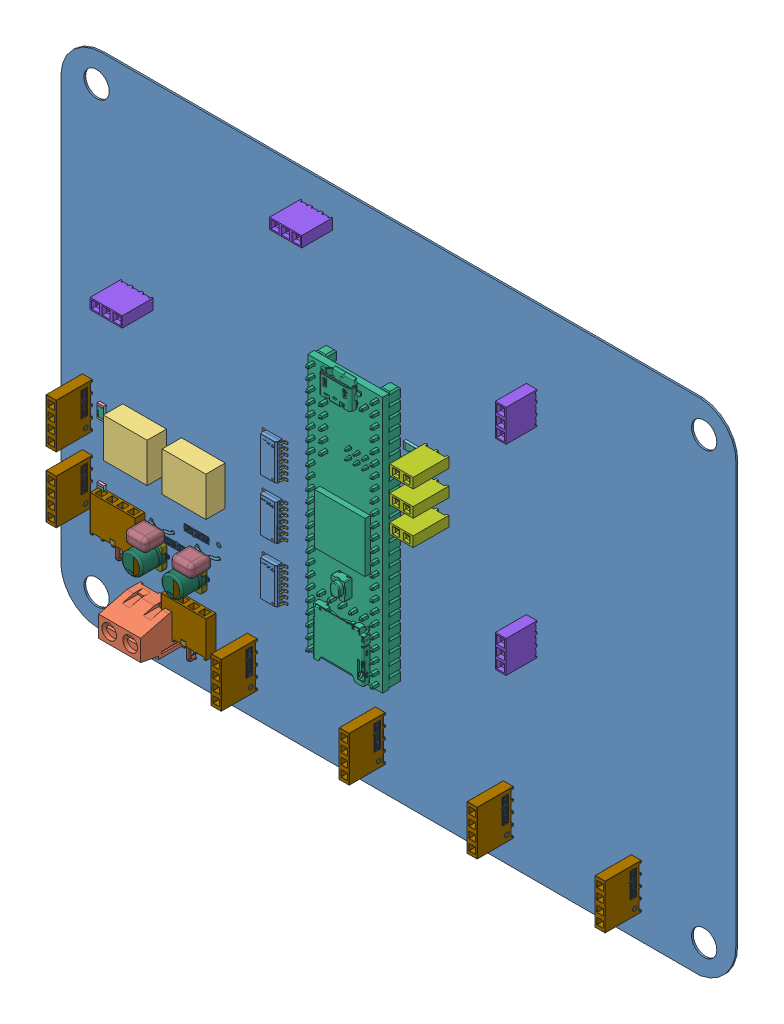
SolidWorks assembly MotherBoardPCB, configuration Default. Lengths in mm.
Overall size (160.64 119 16.7).
180 component instances, 26 part files, 0 mates.
Components (placement in the parent):
- MotherBoardPCB.step-1: MotherBoardPCB.step [Default] at origin size (160.64 119 16.7)
  - Board.step-1: Board.step [Default] at origin size (160.64 119 0.41)
    - Open CASCADE STEP translator 6.8 1.1.1.step-1: Open CASCADE STEP translator 6.8 1.1.1.step [Default] at (0 0 -0.4115) size (160.64 119 0.41)
  - J14.step-1: J14.step [Default] at origin size (10.6 8.2 13.5)
    - c-282836-2-h-3d.step-1: c-282836-2-h-3d.step [Default] at (49.784 31.8411 5) x (1 0 0) z (0 -1 0) size (10.6 13.5 8.2)
  - U6.step-1: U6.step [Default] at origin size (10.4 9.35 4.6)
    - 6221563216.step-1: 6221563216.step [Default] at (45.72 69.847 0) size (10.4 9.35 4.6)
      - Extruded.step-1: Extruded.step [Default] at origin size (10.4 9.35 4.6)
  - R5.step-1: R5.step [Default] at origin size (1.6 3.2 0.65)
    - Res_Samsung_RC3216F111CS_eec.step-1: Res_Samsung_RC3216F111CS_eec.step [Default] at (35.814 70.739 0) x (-1 0 0) z (0 0 1) size (1.6 3.2 0.65)
      - Sides.step-1: Sides.step [Default] at origin size (1.6 3.2 0.65)
      - Core.step-1: Core.step [Default] at origin size (1.6 3.14 0.59)
      - Top.step-1: Top.step [Default] at origin size (1.6 2.3 0.03)
      - Text_Logo.step-1: Text_Logo.step [Default] at (0.8 -1.12 0.65) size (0.2 1.32 0)
  - R4.step-1: R4.step [Default] at origin size (1.6 3.2 0.65)
    - Res_Samsung_RC3216F111CS_eec.step-1: Res_Samsung_RC3216F111CS_eec.step [Default] at (35.814 54.3773 0) x (-1 0 0) z (0 0 1) size (1.6 3.2 0.65)
      - Sides.step-1: Sides.step [Default] at origin size (1.6 3.2 0.65)
      - Core.step-1: Core.step [Default] at origin size (1.6 3.14 0.59)
      - Top.step-1: Top.step [Default] at origin size (1.6 2.3 0.03)
      - Text_Logo.step-1: Text_Logo.step [Default] at (0.8 -1.12 0.65) size (0.2 1.32 0)
  - J13.step-1: J13.step [Default] at origin size (2.41 10.67 11.41)
    - Conn_Samtec_SSW-104-01-G-S-003_eec.step-1: Conn_Samtec_SSW-104-01-G-S-003_eec.step [Default] at (32.131 70.612 0) x (0 1 0) z (0 0 1) size (10.67 2.41 11.41)
      - pins.step-1: pins.step [Default] at origin size (8.41 0.41 5.77)
      - body.step-1: body.step [Default] at origin size (10.67 2.41 8.64)
      - logo.step-1: logo.step [Default] at (-1.27 -1.205 4.32) x (1 0 0) z (0 -1 0) size (8.76 1.82 0)
  - J12.step-1: J12.step [Default] at origin size (2.41 10.67 11.41)
    - Conn_Samtec_SSW-104-01-G-S-003_eec.step-1: Conn_Samtec_SSW-104-01-G-S-003_eec.step [Default] at (32.131 54.991 0) x (0 1 0) z (0 0 1) size (10.67 2.41 11.41)
      - pins.step-1: pins.step [Default] at origin size (8.41 0.41 5.77)
      - body.step-1: body.step [Default] at origin size (10.67 2.41 8.64)
      - logo.step-1: logo.step [Default] at (-1.27 -1.205 4.32) x (1 0 0) z (0 -1 0) size (8.76 1.82 0)
  - D2.step-1: D2.step [Default] at origin size (10.67 12.15 6.58)
    - Diode_Vishay_UF4007-E3-54_eec.step-1: Diode_Vishay_UF4007-E3-54_eec.step [Default] at (40.64 48.641 0) x (1 0 0) z (0 0 1) size (10.67 12.15 6.58)
      - Lead.step-1: Lead.step [Default] at (0 5.438 -3.65) size (0.79 11.66 5.39)
      - body.step-1: body.step [Default] at (0 -2.325 1.35) x (1 0 0) z (0 1 0) size (10.67 2.41 8.64)
      - ring.step-1: ring.step [Default] at (0 -1.7813 1.35) x (0.981351 0 0.192225) z (0 1 0) size (2.7 2.7 1)
  - C4.step-1: C4.step [Default] at origin size (8.76 4.81 10.6)
    - Cap_Kemet_C322C104K5R5TA_eec.step-1: Cap_Kemet_C322C104K5R5TA_eec.step [Default] at (49.911 53.975 0) x (1 0 0) z (0 0 1) size (8.76 4.81 10.6)
      - Package.step-1: Package.step [Default] at origin size (5.09 3.19 4.82)
      - Leads.step-1: Leads.step [Default] at origin size (5.62 0.52 5.79)
      - logo.step-1: logo.step [Default] at origin size (8.76 1.82 0)
  - C3.step-1: C3.step [Default] at origin size (6 5.3 6.1)
    - Cap_Panasonic_Electronic_Components_EEE-FK1H100UR_eec.step-1: Cap_Panasonic_Electronic_Components_EEE-FK1H100UR_eec.step [Default] at (48.641 48.514 0) x (-1 0 0) z (0 0 1) size (6 5.3 6.1)
      - 5_SIZE_CODE_C.step-1: 5_SIZE_CODE_C.step [Default] x (1 0 0) z (0 -1 0) size (6 6.1 5.3)
        - __X2__2022__X0__W__X2__FFFD20AC__X0__SIZE_CODE_C-001.step-1: __X2__2022__X0__W__X2__FFFD20AC__X0__SIZE_CODE_C-001.step [Default] at (0 0.5 0) size (5 5.6 5)
        - __X2__2022__X0__W__X2__FFFD20AC__X0__SIZE_CODE_C-002.step-1: __X2__2022__X0__W__X2__FFFD20AC__X0__SIZE_CODE_C-002.step [Default] at origin size (5.3 1.15 5.3)
        - __X2__2022__X0__W__X2__FFFD20AC__X0__SIZE_CODE_C-003.step-1: __X2__2022__X0__W__X2__FFFD20AC__X0__SIZE_CODE_C-003.step [Default] at (-0.75 0.3 0) size (2.58 1 0.65)
        - __X2__2022__X0__W__X2__FFFD20AC__X0__SIZE_CODE_C-003.step-2: __X2__2022__X0__W__X2__FFFD20AC__X0__SIZE_CODE_C-003.step [Default] at (0.75 0.3 0) x (-1 0 0) z (0 0 -1) size (2.58 1 0.65)
        - 1.step-1: 1.step [Default] at (0 0.499 0) size (3.23 0.2 3.86)
  - U5.step-1: U5.step [Default] at origin size (6 8.65 1.76)
    - IC_Texas_Instruments_OPA4191IDR_eec.step-1: IC_Texas_Instruments_OPA4191IDR_eec.step [Default] at (76.868 56.769 0) x (-1 0 0) z (0 0 1) size (6 8.65 1.76)
      - IC_BODY.step-1: IC_BODY.step [Default] at (0 0 0.25) x (0 -1 0) z (0 0 1) size (8.65 3.9 1.5)
      - circle.step-1: circle.step [Default] at (-1.0199 3.7488 1.751) x (1 0 0) z (0 0 -1) size (0.4 0.4 0)
      - IC_LEG.step-1: IC_LEG.step [Default] at (-3 4.0195 0) x (1 0 0) z (0 -1 0) size (1.15 1.11 0.42)
      - IC_LEG.step-2: IC_LEG.step [Default] at (-3 2.7495 0) x (1 0 0) z (0 -1 0) size (1.15 1.11 0.42)
      - IC_LEG.step-3: IC_LEG.step [Default] at (-3 1.4795 0) x (1 0 0) z (0 -1 0) size (1.15 1.11 0.42)
      - IC_LEG.step-4: IC_LEG.step [Default] at (-3 0.2095 0) x (1 0 0) z (0 -1 0) size (1.15 1.11 0.42)
      - IC_LEG.step-5: IC_LEG.step [Default] at (-3 -1.0605 0) x (1 0 0) z (0 -1 0) size (1.15 1.11 0.42)
      - IC_LEG.step-6: IC_LEG.step [Default] at (-3 -2.3305 0) x (1 0 0) z (0 -1 0) size (1.15 1.11 0.42)
      - IC_LEG.step-7: IC_LEG.step [Default] at (-3 -3.6005 0) x (1 0 0) z (0 -1 0) size (1.15 1.11 0.42)
      - IC_LEG_MIR8.step-1: IC_LEG_MIR8.step [Default] at (3 4.0195 0) x (-1 0 0) z (0 1 0) size (1.15 1.11 0.42)
      - IC_LEG_MIR8.step-2: IC_LEG_MIR8.step [Default] at (3 2.7495 0) x (-1 0 0) z (0 1 0) size (1.15 1.11 0.42)
      - IC_LEG_MIR8.step-3: IC_LEG_MIR8.step [Default] at (3 1.4795 0) x (-1 0 0) z (0 1 0) size (1.15 1.11 0.42)
      - IC_LEG_MIR8.step-4: IC_LEG_MIR8.step [Default] at (3 0.2095 0) x (-1 0 0) z (0 1 0) size (1.15 1.11 0.42)
      - IC_LEG_MIR8.step-5: IC_LEG_MIR8.step [Default] at (3 -1.0605 0) x (-1 0 0) z (0 1 0) size (1.15 1.11 0.42)
      - IC_LEG_MIR8.step-6: IC_LEG_MIR8.step [Default] at (3 -2.3305 0) x (-1 0 0) z (0 1 0) size (1.15 1.11 0.42)
      - IC_LEG_MIR8.step-7: IC_LEG_MIR8.step [Default] at (3 -3.6005 0) x (-1 0 0) z (0 1 0) size (1.15 1.11 0.42)
      - Texas_Instruments.step-1: Texas_Instruments.step [Default] at (-0.0141 -3.2232 1.75) size (3.04 0.71 0.02)
  - U4.step-1: U4.step [Default] at origin size (6 8.65 1.76)
    - IC_Texas_Instruments_OPA4191IDR_eec.step-1: IC_Texas_Instruments_OPA4191IDR_eec.step [Default] at (76.835 69.85 0) x (-1 0 0) z (0 0 1) size (6 8.65 1.76)
      - IC_BODY.step-1: IC_BODY.step [Default] at (0 0 0.25) x (0 -1 0) z (0 0 1) size (8.65 3.9 1.5)
      - circle.step-1: circle.step [Default] at (-1.0199 3.7488 1.751) x (1 0 0) z (0 0 -1) size (0.4 0.4 0)
      - IC_LEG.step-1: IC_LEG.step [Default] at (-3 4.0195 0) x (1 0 0) z (0 -1 0) size (1.15 1.11 0.42)
      - IC_LEG.step-2: IC_LEG.step [Default] at (-3 2.7495 0) x (1 0 0) z (0 -1 0) size (1.15 1.11 0.42)
      - IC_LEG.step-3: IC_LEG.step [Default] at (-3 1.4795 0) x (1 0 0) z (0 -1 0) size (1.15 1.11 0.42)
      - IC_LEG.step-4: IC_LEG.step [Default] at (-3 0.2095 0) x (1 0 0) z (0 -1 0) size (1.15 1.11 0.42)
      - IC_LEG.step-5: IC_LEG.step [Default] at (-3 -1.0605 0) x (1 0 0) z (0 -1 0) size (1.15 1.11 0.42)
      - IC_LEG.step-6: IC_LEG.step [Default] at (-3 -2.3305 0) x (1 0 0) z (0 -1 0) size (1.15 1.11 0.42)
      - IC_LEG.step-7: IC_LEG.step [Default] at (-3 -3.6005 0) x (1 0 0) z (0 -1 0) size (1.15 1.11 0.42)
      - IC_LEG_MIR8.step-1: IC_LEG_MIR8.step [Default] at (3 4.0195 0) x (-1 0 0) z (0 1 0) size (1.15 1.11 0.42)
      - IC_LEG_MIR8.step-2: IC_LEG_MIR8.step [Default] at (3 2.7495 0) x (-1 0 0) z (0 1 0) size (1.15 1.11 0.42)
      - IC_LEG_MIR8.step-3: IC_LEG_MIR8.step [Default] at (3 1.4795 0) x (-1 0 0) z (0 1 0) size (1.15 1.11 0.42)
      - IC_LEG_MIR8.step-4: IC_LEG_MIR8.step [Default] at (3 0.2095 0) x (-1 0 0) z (0 1 0) size (1.15 1.11 0.42)
      - IC_LEG_MIR8.step-5: IC_LEG_MIR8.step [Default] at (3 -1.0605 0) x (-1 0 0) z (0 1 0) size (1.15 1.11 0.42)
      - IC_LEG_MIR8.step-6: IC_LEG_MIR8.step [Default] at (3 -2.3305 0) x (-1 0 0) z (0 1 0) size (1.15 1.11 0.42)
      - IC_LEG_MIR8.step-7: IC_LEG_MIR8.step [Default] at (3 -3.6005 0) x (-1 0 0) z (0 1 0) size (1.15 1.11 0.42)
      - Texas_Instruments.step-1: Texas_Instruments.step [Default] at (-0.0141 -3.2232 1.75) size (3.04 0.71 0.02)
  - U3.step-1: U3.step [Default] at origin size (17.78 61.66 13.85)
    - 6212818880.step-1: 6212818880.step [Default] at (97.79 80.645 0) x (0 -1 0) z (-1 0 0) size (61.66 13.85 17.78)
  - U2.step-1: U2.step [Default] at origin size (6 8.65 1.76)
    - IC_Texas_Instruments_OPA4191IDR_eec.step-1: IC_Texas_Instruments_OPA4191IDR_eec.step [Default] at (76.868 82.296 0) x (-1 0 0) z (0 0 1) size (6 8.65 1.76)
      - IC_BODY.step-1: IC_BODY.step [Default] at (0 0 0.25) x (0 -1 0) z (0 0 1) size (8.65 3.9 1.5)
      - circle.step-1: circle.step [Default] at (-1.0199 3.7488 1.751) x (1 0 0) z (0 0 -1) size (0.4 0.4 0)
      - IC_LEG.step-1: IC_LEG.step [Default] at (-3 4.0195 0) x (1 0 0) z (0 -1 0) size (1.15 1.11 0.42)
      - IC_LEG.step-2: IC_LEG.step [Default] at (-3 2.7495 0) x (1 0 0) z (0 -1 0) size (1.15 1.11 0.42)
      - IC_LEG.step-3: IC_LEG.step [Default] at (-3 1.4795 0) x (1 0 0) z (0 -1 0) size (1.15 1.11 0.42)
      - IC_LEG.step-4: IC_LEG.step [Default] at (-3 0.2095 0) x (1 0 0) z (0 -1 0) size (1.15 1.11 0.42)
      - IC_LEG.step-5: IC_LEG.step [Default] at (-3 -1.0605 0) x (1 0 0) z (0 -1 0) size (1.15 1.11 0.42)
      - IC_LEG.step-6: IC_LEG.step [Default] at (-3 -2.3305 0) x (1 0 0) z (0 -1 0) size (1.15 1.11 0.42)
      - IC_LEG.step-7: IC_LEG.step [Default] at (-3 -3.6005 0) x (1 0 0) z (0 -1 0) size (1.15 1.11 0.42)
      - IC_LEG_MIR8.step-1: IC_LEG_MIR8.step [Default] at (3 4.0195 0) x (-1 0 0) z (0 1 0) size (1.15 1.11 0.42)
      - IC_LEG_MIR8.step-2: IC_LEG_MIR8.step [Default] at (3 2.7495 0) x (-1 0 0) z (0 1 0) size (1.15 1.11 0.42)
      - IC_LEG_MIR8.step-3: IC_LEG_MIR8.step [Default] at (3 1.4795 0) x (-1 0 0) z (0 1 0) size (1.15 1.11 0.42)
      - IC_LEG_MIR8.step-4: IC_LEG_MIR8.step [Default] at (3 0.2095 0) x (-1 0 0) z (0 1 0) size (1.15 1.11 0.42)
      - IC_LEG_MIR8.step-5: IC_LEG_MIR8.step [Default] at (3 -1.0605 0) x (-1 0 0) z (0 1 0) size (1.15 1.11 0.42)
      - IC_LEG_MIR8.step-6: IC_LEG_MIR8.step [Default] at (3 -2.3305 0) x (-1 0 0) z (0 1 0) size (1.15 1.11 0.42)
      - IC_LEG_MIR8.step-7: IC_LEG_MIR8.step [Default] at (3 -3.6005 0) x (-1 0 0) z (0 1 0) size (1.15 1.11 0.42)
      - Texas_Instruments.step-1: Texas_Instruments.step [Default] at (-0.0141 -3.2232 1.75) size (3.04 0.71 0.02)
  - U1.step-1: U1.step [Default] at origin size (10.4 9.35 4.6)
    - 6221563216.step-1: 6221563216.step [Default] at (59.69 69.847 0) size (10.4 9.35 4.6)
      - Extruded.step-1: Extruded.step [Default] at origin size (10.4 9.35 4.6)
  - R3.step-1: R3.step [Default] at origin size (3.2 1.6 0.65)
    - Res_Samsung_RC3216F111CS_eec.step-1: Res_Samsung_RC3216F111CS_eec.step [Default] at (109.474 100.076 0) x (0 -1 0) z (0 0 1) size (1.6 3.2 0.65)
      - Sides.step-1: Sides.step [Default] at origin size (1.6 3.2 0.65)
      - Core.step-1: Core.step [Default] at origin size (1.6 3.14 0.59)
      - Top.step-1: Top.step [Default] at origin size (1.6 2.3 0.03)
      - Text_Logo.step-1: Text_Logo.step [Default] at (0.8 -1.12 0.65) size (0.2 1.32 0)
  - R2.step-1: R2.step [Default] at origin size (3.2 1.6 0.65)
    - Res_Samsung_RC3216F111CS_eec.step-1: Res_Samsung_RC3216F111CS_eec.step [Default] at (109.474 94.996 0) x (0 -1 0) z (0 0 1) size (1.6 3.2 0.65)
      - Sides.step-1: Sides.step [Default] at origin size (1.6 3.2 0.65)
      - Core.step-1: Core.step [Default] at origin size (1.6 3.14 0.59)
      - Top.step-1: Top.step [Default] at origin size (1.6 2.3 0.03)
      - Text_Logo.step-1: Text_Logo.step [Default] at (0.8 -1.12 0.65) size (0.2 1.32 0)
  - R1.step-1: R1.step [Default] at origin size (3.2 1.6 0.65)
    - Res_Samsung_RC3216F111CS_eec.step-1: Res_Samsung_RC3216F111CS_eec.step [Default] at (109.474 89.789 0) x (0 -1 0) z (0 0 1) size (1.6 3.2 0.65)
      - Sides.step-1: Sides.step [Default] at origin size (1.6 3.2 0.65)
      - Core.step-1: Core.step [Default] at origin size (1.6 3.14 0.59)
      - Top.step-1: Top.step [Default] at origin size (1.6 2.3 0.03)
      - Text_Logo.step-1: Text_Logo.step [Default] at (0.8 -1.12 0.65) size (0.2 1.32 0)
  - J11.step-1: J11.step [Default] at origin size (5.59 2.41 13.44)
    - SSW-102-02-X-S.step-1: SSW-102-02-X-S.step [Default] at (115.3161 89.1541 0) x (0 1 0) z (1 0 0) size (2.41 13.44 5.59)
  - J10.step-1: J10.step [Default] at origin size (5.59 2.41 13.44)
    - SSW-102-02-X-S.step-1: SSW-102-02-X-S.step [Default] at (115.3161 95.1866 0) x (0 1 0) z (1 0 0) size (2.41 13.44 5.59)
  - J9.step-1: J9.step [Default] at origin size (5.59 2.41 13.44)
    - SSW-102-02-X-S.step-1: SSW-102-02-X-S.step [Default] at (115.3161 101.2191 0) x (0 1 0) z (1 0 0) size (2.41 13.44 5.59)
  - J8.step-1: J8.step [Default] at origin size (2.41 10.67 11.41)
    - Conn_Samtec_SSW-104-01-G-S-003_eec.step-1: Conn_Samtec_SSW-104-01-G-S-003_eec.step [Default] at (162.687 36.83 0) x (0 1 0) z (0 0 1) size (10.67 2.41 11.41)
      - pins.step-1: pins.step [Default] at origin size (8.41 0.41 5.77)
      - body.step-1: body.step [Default] at origin size (10.67 2.41 8.64)
      - logo.step-1: logo.step [Default] at (-1.27 -1.205 4.32) x (1 0 0) z (0 -1 0) size (8.76 1.82 0)
  - J7.step-1: J7.step [Default] at origin size (2.41 10.67 11.41)
    - Conn_Samtec_SSW-104-01-G-S-003_eec.step-1: Conn_Samtec_SSW-104-01-G-S-003_eec.step [Default] at (132.2493 36.83 0) x (0 1 0) z (0 0 1) size (10.67 2.41 11.41)
      - pins.step-1: pins.step [Default] at origin size (8.41 0.41 5.77)
      - body.step-1: body.step [Default] at origin size (10.67 2.41 8.64)
      - logo.step-1: logo.step [Default] at (-1.27 -1.205 4.32) x (1 0 0) z (0 -1 0) size (8.76 1.82 0)
  - J6.step-1: J6.step [Default] at origin size (2.41 10.67 11.41)
    - Conn_Samtec_SSW-104-01-G-S-003_eec.step-1: Conn_Samtec_SSW-104-01-G-S-003_eec.step [Default] at (101.8117 36.83 0) x (0 1 0) z (0 0 1) size (10.67 2.41 11.41)
      - pins.step-1: pins.step [Default] at origin size (8.41 0.41 5.77)
      - body.step-1: body.step [Default] at origin size (10.67 2.41 8.64)
      - logo.step-1: logo.step [Default] at (-1.27 -1.205 4.32) x (1 0 0) z (0 -1 0) size (8.76 1.82 0)
  - J5.step-1: J5.step [Default] at origin size (2.41 10.67 11.41)
    - Conn_Samtec_SSW-104-01-G-S-003_eec.step-1: Conn_Samtec_SSW-104-01-G-S-003_eec.step [Default] at (71.374 36.83 0) x (0 1 0) z (0 0 1) size (10.67 2.41 11.41)
      - pins.step-1: pins.step [Default] at origin size (8.41 0.41 5.77)
      - body.step-1: body.step [Default] at origin size (10.67 2.41 8.64)
      - logo.step-1: logo.step [Default] at (-1.27 -1.205 4.32) x (1 0 0) z (0 -1 0) size (8.76 1.82 0)
  - J4.step-1: J4.step [Default] at origin size (7.62 2.54 10.46)
    - BCS-103-X-S-TE.step-1: BCS-103-X-S-TE.step [Default] at (86.6139 136.5249 0) x (-1 0 0) z (0 1 0) size (7.62 10.46 2.54)
  - J3.step-1: J3.step [Default] at origin size (2.54 7.62 10.46)
    - BCS-103-X-S-TE.step-1: BCS-103-X-S-TE.step [Default] at (137.7949 75.3111 0) x (0 1 0) z (1 0 0) size (7.62 10.46 2.54)
  - J2.step-1: J2.step [Default] at origin size (2.54 7.62 10.46)
    - BCS-103-X-S-TE.step-1: BCS-103-X-S-TE.step [Default] at (137.7949 122.9361 0) x (0 1 0) z (1 0 0) size (7.62 10.46 2.54)
  - J1.step-1: J1.step [Default] at origin size (7.62 2.54 10.46)
    - BCS-103-X-S-TE.step-1: BCS-103-X-S-TE.step [Default] at (43.9419 98.6789 0) x (-1 0 0) z (0 1 0) size (7.62 10.46 2.54)
  - D1.step-1: D1.step [Default] at origin size (10.67 12.15 6.58)
    - Diode_Vishay_UF4007-E3-54_eec.step-1: Diode_Vishay_UF4007-E3-54_eec.step [Default] at (57.531 36.345 0) x (1 0 0) z (0 0 1) size (10.67 12.15 6.58)
      - Lead.step-1: Lead.step [Default] at (0 5.438 -3.65) size (0.79 11.66 5.39)
      - body.step-1: body.step [Default] at (0 -2.325 1.35) x (1 0 0) z (0 1 0) size (10.67 2.41 8.64)
      - ring.step-1: ring.step [Default] at (0 -1.7813 1.35) x (0.981351 0 0.192225) z (0 1 0) size (2.7 2.7 1)
  - C2.step-1: C2.step [Default] at origin size (8.76 4.81 10.6)
    - Cap_Kemet_C322C104K5R5TA_eec.step-1: Cap_Kemet_C322C104K5R5TA_eec.step [Default] at (60.833 54.102 0) x (-1 0 0) z (0 0 1) size (8.76 4.81 10.6)
      - Package.step-1: Package.step [Default] at origin size (5.09 3.19 4.82)
      - Leads.step-1: Leads.step [Default] at origin size (5.62 0.52 5.79)
      - logo.step-1: logo.step [Default] at origin size (8.76 1.82 0)
  - C1.step-1: C1.step [Default] at origin size (6 5.3 6.1)
    - Cap_Panasonic_Electronic_Components_EEE-FK1H100UR_eec.step-1: Cap_Panasonic_Electronic_Components_EEE-FK1H100UR_eec.step [Default] at (58.166 48.641 0) x (-1 0 0) z (0 0 1) size (6 5.3 6.1)
      - 5_SIZE_CODE_C.step-1: 5_SIZE_CODE_C.step [Default] x (1 0 0) z (0 -1 0) size (6 6.1 5.3)
        - __X2__2022__X0__W__X2__FFFD20AC__X0__SIZE_CODE_C-001.step-1: __X2__2022__X0__W__X2__FFFD20AC__X0__SIZE_CODE_C-001.step [Default] at (0 0.5 0) size (5 5.6 5)
        - __X2__2022__X0__W__X2__FFFD20AC__X0__SIZE_CODE_C-002.step-1: __X2__2022__X0__W__X2__FFFD20AC__X0__SIZE_CODE_C-002.step [Default] at origin size (5.3 1.15 5.3)
        - __X2__2022__X0__W__X2__FFFD20AC__X0__SIZE_CODE_C-003.step-1: __X2__2022__X0__W__X2__FFFD20AC__X0__SIZE_CODE_C-003.step [Default] at (-0.75 0.3 0) size (2.58 1 0.65)
        - __X2__2022__X0__W__X2__FFFD20AC__X0__SIZE_CODE_C-003.step-2: __X2__2022__X0__W__X2__FFFD20AC__X0__SIZE_CODE_C-003.step [Default] at (0.75 0.3 0) x (-1 0 0) z (0 0 -1) size (2.58 1 0.65)
        - 1.step-1: 1.step [Default] at (0 0.499 0) size (3.23 0.2 3.86)
